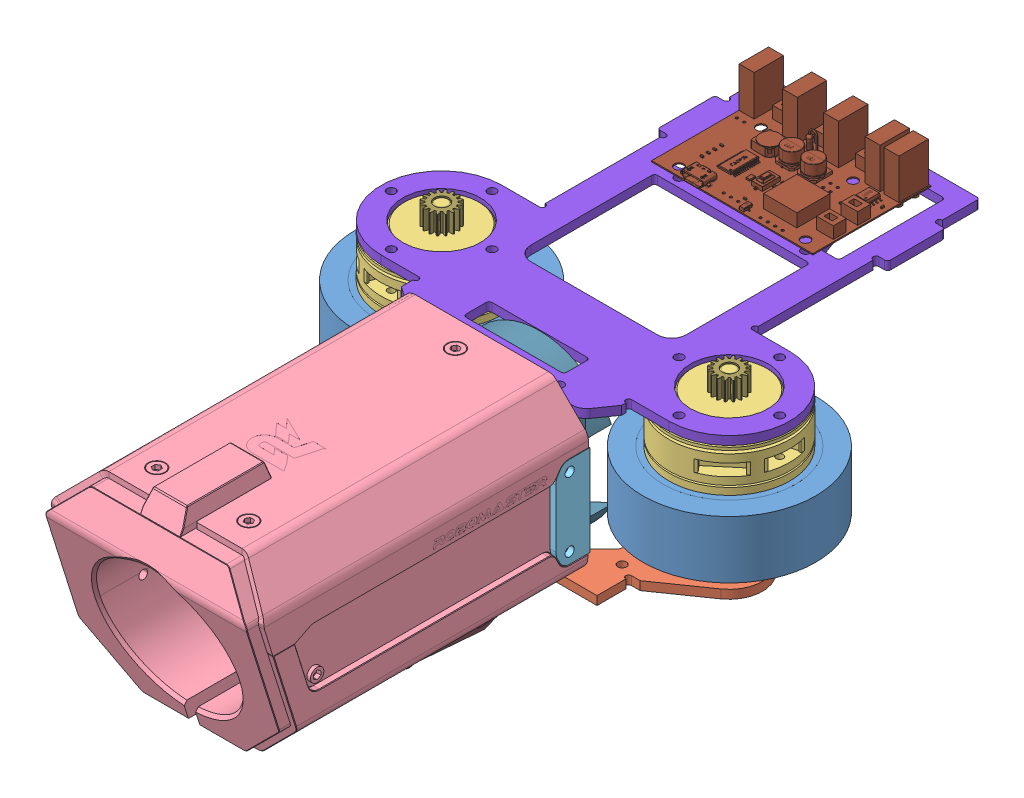
SolidWorks assembly pitch轴大发射, configuration 默认. Lengths in mm.
Overall size (160 95.03 252.73).
27 component instances, 14 part files, 57 mates.
Components (placement in the parent):
- 摩擦轮-1: 摩擦轮 [默认] at origin size (160 20 60)
- 发射机构底板-1: 发射机构底板 [默认] at (0 -28 0) x (-1 0 0) z (0 0 -1) size (123 3 59.75)
- M3508电机无减速箱-1: M3508电机无减速箱 [默认] at (50 61 0) x (-0.707107 0 0.707107) z (-0.707107 0 -0.707107) size (42 43.4 42)
- RM2019裁判系统测速模块SM11-1: RM2019裁判系统测速模块SM11 [默认] at (21.5261 -69.6659 -28.7637) size (74 74 119.73)
- 测速模块卡板-1: 测速模块卡板 [默认] at (21.5261 -69.6659 -28.7637) size (2 31.6 11.8)
- 摩擦轴承连接法兰-1: 摩擦轴承连接法兰 [默认] at (50 -10 0) x (-1 0 0) z (0 0 1) size (27.52 19.2 26)
- 法兰轴承F6700zz-10x15x4-16.5x0.8-1: 法兰轴承F6700zz-10x15x4-16.5x0.8 [默认] at (50 -28.2 0) x (0 1 0) z (-0.223049 0 -0.974807) size (4 16.5 16.5)
- 摩擦轮安装板-1: 摩擦轮安装板 [默认] at (0 25 0) x (-1 0 0) z (0 0 -1) size (142 3 133)
- 法兰轴承F6700zz-10x15x4-16.5x0.8-2: 法兰轴承F6700zz-10x15x4-16.5x0.8 [默认] at (-50 -28.2 0) x (0 1 0) z (-0.223049 0 0.974807) size (4 16.5 16.5)
- 摩擦轴承连接法兰-2: 摩擦轴承连接法兰 [默认] at (-50 -10 0) x (-1 0 0) z (0 0 1) size (27.52 19.2 26)
- M3508电机无减速箱-3: M3508电机无减速箱 [默认] at (-50 61 0) x (-0.707107 0 -0.707107) z (0.707107 0 -0.707107) size (42 43.4 42)
- hexagon socket head cap screws gb-3: hexagon socket head cap screws gb [GB_FASTENER_SCREWS_HSHCS M3X6-C] at (43.5 -10.1 0) x (0 1 0) z (0.546944 0 -0.837169) size (9 5.5 5.5)
- hexagon socket head cap screws gb-4: hexagon socket head cap screws gb [GB_FASTENER_SCREWS_HSHCS M3X6-C] at (56.5 -10.1 0) x (0 1 0) z (0.546944 0 -0.837169) size (9 5.5 5.5)
- hexagon socket head cap screws gb-5: hexagon socket head cap screws gb [GB_FASTENER_SCREWS_HSHCS M3X6-C] at (38.7417 -15 6.5) x (0 1 0) z (0.524684 0 -0.851297) size (9 5.5 5.5)
- hexagon socket head cap screws gb-6: hexagon socket head cap screws gb [GB_FASTENER_SCREWS_HSHCS M3X6-C] at (61.2583 -15 6.5) x (0 1 0) z (0.546944 0 -0.837169) size (9 5.5 5.5)
- hexagon socket head cap screws gb-7: hexagon socket head cap screws gb [GB_FASTENER_SCREWS_HSHCS M3X6-C] at (50 -15 -13) x (0 1 0) z (0.546944 0 -0.837169) size (9 5.5 5.5)
- 镜向测速模块固定打印件-2: 镜向测速模块固定打印件 [默认] at (-21.5261 -69.6659 -28.7637) x (-1 0 0) z (0 0 -1) size (2 31.6 11.8)
- hexagon socket head cap screws gb-8: hexagon socket head cap screws gb [GB_FASTENER_SCREWS_HSHCS M3X6-C] at (-61.2583 -15 6.5) x (0 1 0) z (0.546944 0 0.837169) size (9 5.5 5.5)
- hexagon socket head cap screws gb-9: hexagon socket head cap screws gb [GB_FASTENER_SCREWS_HSHCS M3X6-C] at (-38.7417 -15 6.5) x (0 1 0) z (0.524684 0 0.851297) size (9 5.5 5.5)
- hexagon socket head cap screws gb-10: hexagon socket head cap screws gb [GB_FASTENER_SCREWS_HSHCS M3X6-C] at (-50 -15 -13) x (0 1 0) z (0.546944 0 0.837169) size (9 5.5 5.5)
- hexagon socket head cap screws gb-11: hexagon socket head cap screws gb [GB_FASTENER_SCREWS_HSHCS M3X6-C] at (-43.5 -10.1 0) x (0 1 0) z (0.546944 0 0.837169) size (9 5.5 5.5)
- hexagon socket head cap screws gb-12: hexagon socket head cap screws gb [GB_FASTENER_SCREWS_HSHCS M3X6-C] at (-56.5 -10.1 0) x (0 1 0) z (0.546944 0 0.837169) size (9 5.5 5.5)
- Hero_Master-1: Hero_Master [默认] at (28 31.4115 -92) x (-1 0 0.000001) z (0 1 0) size (56 41.25 17)
- spur gear_gb-1: spur gear_gb [GB - Spur gear 0.6M 16T 20PA 6.5FW ---S16A75H50L5.0N] at (50 33.5 0) x (0 -1 0) z (0 0 1) size (6.5 10.64 10.64)
- spur gear_gb-2: spur gear_gb [GB - Spur gear 0.6M 16T 20PA 6.5FW ---S16A75H50L5.0N] at (-50 33.5 0) x (0 -1 0) z (0 0 -1) size (6.5 10.64 10.64)
- RoboMaster 红点激光器-1: RoboMaster 红点激光器 [默认] at (20.4617 -46.413 101.4662) x (-1 0 0) z (0 0 1) size (25 20.86 51.36)
- 炮管-1: 炮管 [默认] at (0 0 33) size (50 55.5 52)
Mates (geometry in assembly coordinates):
- 重合1: coincident: plane of 摩擦轮安装板-1 through (-50 25 0) normal (0 -1 0); plane of M3508电机无减速箱-1 through (79.6255 25 0) normal (0 1 0)
- 同心1: concentric: cylinder of M3508电机无减速箱-1 through (50 26.5 0) axis (0 -1 0) radius 13.4; cylinder of 摩擦轮安装板-1 through (50 28 0) axis (0 -1 0) radius 13.5
- 同心2: concentric: cylinder of M3508电机无减速箱-1 through (50 10 -17.5) axis (0 1 0) radius 1.25; cylinder of 摩擦轮安装板-1 through (50 28 -17.5) axis (0 -1 0) radius 1.5
- 重合3: coincident: plane of 摩擦轮-1 through (0 0 0) normal (1 0 0); plane of assembly through (0 0 0) normal (1 0 0)
- 同心7: concentric: cylinder of RM2019裁判系统测速模块SM11-1 through (27 -7 42.5) axis (1 0 0) radius 2; cylinder of 测速模块卡板-1 through (71.176 -7 42.5) axis (-1 0 0) radius 1.6
- 同心8: concentric: cylinder of RM2019裁判系统测速模块SM11-1 through (35 17 42.5) axis (-1 0 0) radius 1.6; cylinder of 测速模块卡板-1 through (71.176 17 42.5) axis (-1 0 0) radius 1.6
- 重合10: coincident: plane of RM2019裁判系统测速模块SM11-1 through (35 13.152 137) normal (1 0 0); plane of 测速模块卡板-1 through (35 -7 42.5279) normal (-1 0 0)
- 重合11: coincident: plane of 摩擦轮-1 through (0 0 0) normal (0 0 1); plane of assembly through (0 0 0) normal (0 0 1)
- 重合12: coincident: plane of 摩擦轮-1 through (0 0 0) normal (0 1 0); plane of assembly through (0 0 0) normal (0 1 0)
- 重合13: coincident: plane of 发射机构底板-1 through (50 -25 0) normal (0 1 0); plane of 摩擦轮-1 through (-25 -25 -70.7107) normal (0 -1 0)
- 同心9: concentric: cylinder of 发射机构底板-1 through (19.5 -25 -14.25) axis (0 -1 0) radius 1.5; cylinder of 摩擦轮-1 through (19.5 -25 -14.25) axis (0 1 0) radius 1.5
- 同心10: concentric: cylinder of 发射机构底板-1 through (19.5 -25 14.25) axis (0 -1 0) radius 1.5; cylinder of 摩擦轮-1 through (19.5 -25 14.25) axis (0 1 0) radius 1.5
- 同心11: concentric: cylinder of RM2019裁判系统测速模块SM11-1 through (8 -28 71.3) axis (0 -1 0) radius 1.9; cylinder of 摩擦轮-1 through (8 -36 71.3) axis (0 1 0) radius 1.5
- 同心12: concentric: cylinder of 摩擦轮-1 through (8 -36 41.3) axis (0 1 0) radius 1.5; cylinder of RM2019裁判系统测速模块SM11-1 through (8 -28 41.3) axis (0 -1 0) radius 1.9
- 同心16: concentric: cylinder of 摩擦轴承连接法兰-1 through (50 -28.9 0) axis (0 -1 0) radius 10.5; cylinder of 摩擦轮-1 through (50 37 0) axis (0 1 0) radius 10.5
- 同心17: concentric: cylinder of 摩擦轴承连接法兰-1 through (50 -9 -13) axis (0 -1 0) radius 1.5; cylinder of 摩擦轮-1 through (50 -10 -13) axis (0 1 0) radius 1.25
- 重合15: coincident: plane of 摩擦轴承连接法兰-1 through (50 -10 0) normal (0 1 0); plane of 摩擦轮-1 through (0 -10 0) normal (0 -1 0)
- 同心19: concentric: cylinder of 摩擦轴承连接法兰-1 through (50 -28.9 0) axis (0 -1 0) radius 5; cylinder of 法兰轴承F6700zz-10x15x4-16.5x0.8-1 through (50 -28.2 0) axis (0 -1 0) radius 5
- 重合17: coincident: plane of 摩擦轴承连接法兰-1 through (50 -24.2 0) normal (0 -1 0); plane of 法兰轴承F6700zz-10x15x4-16.5x0.8-1 through (54.874 -24.2 -1.1152) normal (0 1 0)
- 同心20: concentric: cylinder of 摩擦轮-1 through (19.5 -25 14.25) axis (0 1 0) radius 1.5; cylinder of 摩擦轮安装板-1 through (19.5 28 14.25) axis (0 -1 0) radius 1.5
- 同心21: concentric: cylinder of 摩擦轮-1 through (19.5 -25 -14.25) axis (0 1 0) radius 1.5; cylinder of 摩擦轮安装板-1 through (19.5 28 -14.25) axis (0 -1 0) radius 1.5
- 重合18: coincident: plane of 摩擦轮-1 through (0 25 -22.5) normal (0 1 0); plane of 摩擦轮安装板-1 through (-50 25 0) normal (0 -1 0)
- 同心32: concentric: cylinder of 摩擦轮-1 through (0 0 -22.5) axis (0 0 1) radius 22.75; cylinder of RM2019裁判系统测速模块SM11-1 through (0 0 153.0007) axis (0 0 -1) radius 24.25
- 同心33: concentric: cylinder of M3508电机无减速箱-3 through (-50 26.5 0) axis (0 -1 0) radius 13.4; cylinder of 摩擦轮安装板-1 through (-50 28 0) axis (0 -1 0) radius 13.5
- 同心34: concentric: cylinder of M3508电机无减速箱-3 through (-50 21.2 17.5) axis (0 1 0) radius 1.25; cylinder of 摩擦轮安装板-1 through (-50 28 17.5) axis (0 -1 0) radius 1.5
- 重合22: coincident: plane of 摩擦轮安装板-1 through (-50 25 0) normal (0 -1 0); plane of M3508电机无减速箱-3 through (-50 25 29.6255) normal (0 1 0)
- 同心39: concentric: cylinder of 摩擦轮-1 through (43.5 10 0) axis (0 -1 0) radius 1.5; cylinder of hexagon socket head cap screws gb-3 through (43.5 -1.1 0) axis (0 -1 0) radius 1.5
- 重合25: coincident: plane of 摩擦轮-1 through (0 -7.1 0) normal (0 -1 0); plane of hexagon socket head cap screws gb-3 through (43.5 -7.1 0) normal (0 1 0)
- 同心40: concentric: cylinder of 摩擦轮-1 through (56.5 10 0) axis (0 -1 0) radius 1.5; cylinder of hexagon socket head cap screws gb-4 through (56.5 -1.1 0) axis (0 -1 0) radius 1.5
- 重合26: coincident: plane of 摩擦轮-1 through (0 -7.1 0) normal (0 -1 0); plane of hexagon socket head cap screws gb-4 through (56.5 -7.1 0) normal (0 1 0)
- 同心41: concentric: cylinder of 摩擦轴承连接法兰-1 through (38.7417 -9 6.5) axis (0 -1 0) radius 1.5; cylinder of hexagon socket head cap screws gb-5 through (38.7417 -6 6.5) axis (0 -1 0) radius 1.5
- 重合27: coincident: plane of 摩擦轴承连接法兰-1 through (50 -12 0) normal (0 -1 0); plane of hexagon socket head cap screws gb-5 through (38.7417 -12 6.5) normal (0 1 0)
- 同心42: concentric: cylinder of 摩擦轴承连接法兰-1 through (61.2583 -9 6.5) axis (0 -1 0) radius 1.5; cylinder of hexagon socket head cap screws gb-6 through (61.2583 -6 6.5) axis (0 -1 0) radius 1.5
- 重合28: coincident: plane of 摩擦轴承连接法兰-1 through (50 -12 0) normal (0 -1 0); plane of hexagon socket head cap screws gb-6 through (61.2583 -12 6.5) normal (0 1 0)
- 同心43: concentric: cylinder of 摩擦轴承连接法兰-1 through (50 -9 -13) axis (0 -1 0) radius 1.5; cylinder of hexagon socket head cap screws gb-7 through (50 -6 -13) axis (0 -1 0) radius 1.5
- 重合29: coincident: plane of 摩擦轴承连接法兰-1 through (50 -12 0) normal (0 -1 0); plane of hexagon socket head cap screws gb-7 through (50 -12 -13) normal (0 1 0)
- 距离1: distance = 3 mm: plane of Hero_Master-1 through (28 31 -92) normal (0 -1 0); plane of 摩擦轮安装板-1 through (-50 28 0) normal (0 1 0)
- 同心84: concentric: cylinder of Hero_Master-1 through (22.5 31 -54) axis (0 -1 0) radius 1.6; cylinder of 摩擦轮安装板-1 through (22.5 28 -54) axis (0 -1 0) radius 1.5
- 同心85: concentric: cylinder of Hero_Master-1 through (13 31 -80) axis (0 -1 0) radius 1.6; cylinder of 摩擦轮安装板-1 through (13 28 -80) axis (0 -1 0) radius 1.5
- 重合62: coincident: plane of 摩擦轮安装板-1 through (28 28 -60) normal (1 0 0); plane of Hero_Master-1 through (28 31 -44.4825) normal (1 0 0)
- 同心86: concentric: cylinder of M3508电机无减速箱-1 through (50 32.8 0) axis (0 -1 0) radius 2.5; cylinder of spur gear_gb-1 through (50 -16.5001 0) axis (0 1 0) radius 2.5
- 重合65: coincident: plane of M3508电机无减速箱-1 through (68.4623 27 0) normal (0 1 0); plane of spur gear_gb-1 through (50 27 0) normal (0 -1 0)
- 同心87: concentric: cylinder of RoboMaster 红点激光器-1 through (-8 -32 71.2993) axis (0 1 0) radius 1.25; cylinder of RM2019裁判系统测速模块SM11-1 through (-8 -28 71.2993) axis (0 -1 0) radius 1.9
- 同心88: concentric: cylinder of RM2019裁判系统测速模块SM11-1 through (8 -28 71.2993) axis (0 -1 0) radius 1.9; cylinder of RoboMaster 红点激光器-1 through (8 -32 71.2993) axis (0 1 0) radius 1.25
- 重合67: coincident: plane of RM2019裁判系统测速模块SM11-1 through (-18.8284 -32 200.6578) normal (0 -1 0); plane of RoboMaster 红点激光器-1 through (0 -32 56.2993) normal (0 -1 0)
- 同心89: concentric: cylinder of RM2019裁判系统测速模块SM11-1 through (0 0 153) axis (0 0 -1) radius 24.25; cylinder of 炮管-1 through (0 0 68) axis (0 0 -1) radius 24.25
- 重合68: coincident: plane of RM2019裁判系统测速模块SM11-1 through (0 0 33) normal (0 0 -1); plane of 炮管-1 through (0 0 33) normal (0 0 1)
- 同心90: concentric: cylinder of 摩擦轮-1 through (50 37 0) axis (0 1 0) radius 21; cylinder of 摩擦轮安装板-1 through (50 28 0) axis (0 -1 0) radius 13.5
- 同心91: concentric: cylinder of 摩擦轮-1 through (-50 37 0) axis (0 1 0) radius 21; cylinder of 摩擦轮安装板-1 through (-50 28 0) axis (0 -1 0) radius 13.5
- 重合70: coincident: plane of 摩擦轮-1 through (0 -5.1 0) normal (0 1 0); plane of M3508电机无减速箱-1 through (50 -5.1 -26.1549) normal (0 -1 0)
- 同心92: concentric: cylinder of 发射机构底板-1 through (50 -25 0) axis (0 -1 0) radius 7.6; cylinder of 法兰轴承F6700zz-10x15x4-16.5x0.8-1 through (50 -28.2 0) axis (0 -1 0) radius 7.5
- 同心94: concentric: cylinder of 发射机构底板-1 through (-50 -25 0) axis (0 -1 0) radius 7.6; cylinder of 法兰轴承F6700zz-10x15x4-16.5x0.8-2 through (-50 -28.2 0) axis (0 -1 0) radius 7.5
- 重合71: coincident: plane of 发射机构底板-1 through (50 -25 0) normal (0 1 0); plane of 法兰轴承F6700zz-10x15x4-16.5x0.8-1 through (58.0422 -25 -1.8402) normal (0 -1 0)
- 同心95: concentric: cylinder of 摩擦轮安装板-1 through (20 28 29) axis (0 -1 0) radius 1.5; cylinder of 炮管-1 through (20 25 29) axis (0 1 0) radius 1.25
- 同心96: concentric: cylinder of 摩擦轮安装板-1 through (-20 28 29) axis (0 -1 0) radius 1.5; cylinder of 炮管-1 through (-20 25 29) axis (0 1 0) radius 1.25
- 重合72: coincident: plane of 摩擦轮安装板-1 through (-50 25 0) normal (0 -1 0); plane of 炮管-1 through (25 25 25) normal (0 1 0)
- 平行5: parallel: plane of 发射机构底板-1 through (50 -28 0) normal (0 -1 0); plane of RM2019裁判系统测速模块SM11-1 through (18.8284 -32 200.6578) normal (0 -1 0)
